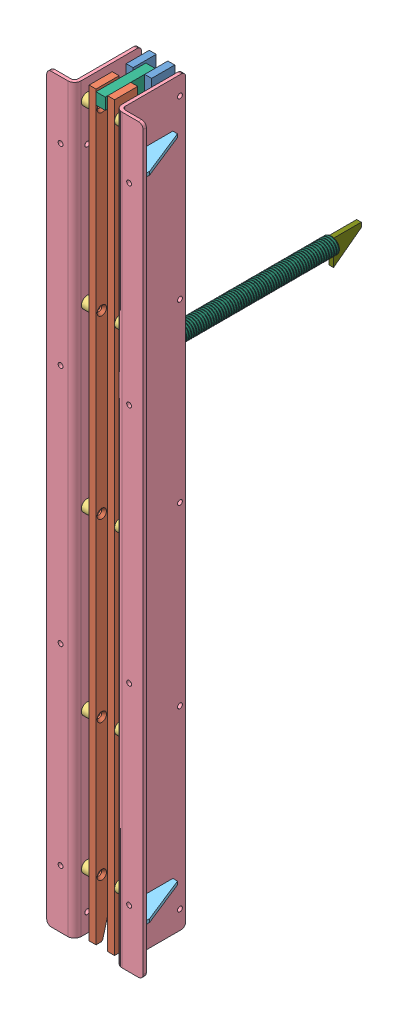
SolidWorks assembly GE-17046_ASM_34_ASM, configuration Default. Lengths in mm.
Overall size (132.08 1016 362.08).
57 component instances, 16 part files, 0 mates.
Components (placement in the parent):
- GE-17052_ASM_16_ASM-1: GE-17052_ASM_16_ASM [Default] at origin size (58.1 1016 92.08)
  - GE-17053_21-1: GE-17053_21 [Default] at origin size (9.53 1016 31.75)
  - GE-17054_26-1: GE-17054_26 [Default] at (9.525 1016 50.8) x (-1 0 0) z (0 0 1) size (9.53 1016 31.75)
  - GE-17057_10-1: GE-17057_10 [Default] at (20.0025 990.6 58.7375) x (-1 0 0) z (0 0 1) size (10.48 15.88 15.88)
  - GE-17057_10-2: GE-17057_10 [Default] at (9.525 25.4 -7.9375) size (10.48 15.88 15.88)
  - GE-17057_10-3: GE-17057_10 [Default] at (20.0025 749.3 58.7375) x (-1 0 0) z (0 0 1) size (10.48 15.88 15.88)
  - GE-17057_10-4: GE-17057_10 [Default] at (9.525 266.7 -7.9375) size (10.48 15.88 15.88)
  - GE-17057_10-5: GE-17057_10 [Default] at (20.0025 508 58.7375) x (-1 0 0) z (0 0 1) size (10.48 15.88 15.88)
  - GE-17057_10-6: GE-17057_10 [Default] at (9.525 508 -7.9375) size (10.48 15.88 15.88)
  - GE-17057_10-7: GE-17057_10 [Default] at (20.0025 266.7 58.7375) x (-1 0 0) z (0 0 1) size (10.48 15.88 15.88)
  - GE-17057_10-8: GE-17057_10 [Default] at (9.525 749.3 -7.9375) size (10.48 15.88 15.88)
  - GE-17057_10-9: GE-17057_10 [Default] at (20.0025 79.375 58.7375) x (-1 0 0) z (0 0 1) size (10.48 15.88 15.88)
  - GE-17057_10-10: GE-17057_10 [Default] at (9.525 990.6 -7.9375) size (10.48 15.88 15.88)
  - GE-17058_ASM_11_ASM-1: GE-17058_ASM_11_ASM [Default] at (20.0025 508 76.2) x (1 0 0) z (0 0 -1) size (38.1 1016 92.08)
    - GE-17058-01_19-1: GE-17058-01_19 [Default] at origin size (38.1 1016 92.08)
    - GE-17058-02_4-1: GE-17058-02_4 [Default] at (4.5542 -445.8792 4.5542) size (31.75 4.55 69.85)
    - GE-17058-02_4-2: GE-17058-02_4 [Default] at (4.5542 441.325 4.5542) size (31.75 4.55 69.85)
- GE-17047_ASM_25_ASM-1: GE-17047_ASM_25_ASM [Default] at (-1.5875 1014.4125 25.4) x (-1 0 0) z (0 0 1) size (49.23 520.7 354.14)
  - GE-17048_24-1: GE-17048_24 [Default] at origin size (12.7 520.7 85.73)
  - GE-17051_2-1: GE-17051_2 [Default] at (15.4686 179.3875 0) x (-1 0 0) z (0 0 1) size (2.77 9.53 9.53)
  - GE-17051_2-2: GE-17051_2 [Default] at (0 179.3875 0) x (-1 0 0) z (0 0 1) size (2.77 9.53 9.53)
  - GE-17050_3-1: GE-17050_3 [Default] at (15.4686 179.3875 0) size (4.98 15.88 15.88)
  - GE-17050_3-2: GE-17050_3 [Default] at (-7.747 179.3875 0) size (4.98 15.88 15.88)
  - HW-00501_2-1: HW-00501_2 [Default] at (23.7998 179.3875 0) x (0 1 0) z (1 0 0) size (11.17 11.22 39.58)
  - HW-00502_2_ASM-1: HW-00502_2_ASM [Default] at (-4.9784 179.3875 0) x (0 1 0) z (0 0 1) size (11.11 5.36 12.83)
    - MANIFOLD_SOLID_BREP_212996-1: MANIFOLD_SOLID_BREP_212996 [Default] at origin size (10.65 1.02 10.65)
    - MANIFOLD_SOLID_BREP_214924-1: MANIFOLD_SOLID_BREP_214924 [Default] at origin size (11.11 5.36 12.83)
  - GE-17051_2-3: GE-17051_2 [Default] at (15.4686 52.3875 0) x (-1 0 0) z (0 0 1) size (2.77 9.53 9.53)
  - GE-17051_2-4: GE-17051_2 [Default] at (0 52.3875 0) x (-1 0 0) z (0 0 1) size (2.77 9.53 9.53)
  - GE-17050_3-3: GE-17050_3 [Default] at (15.4686 52.3875 0) size (4.98 15.88 15.88)
  - GE-17050_3-4: GE-17050_3 [Default] at (-7.747 52.3875 0) size (4.98 15.88 15.88)
  - GE-17056_5-1: GE-17056_5 [Default] at (20.447 52.3875 0) size (4.76 9.53 9.53)
  - GE-17056_5-2: GE-17056_5 [Default] at (-12.5095 52.3875 0) size (4.76 9.53 9.53)
  - HW-00502_2_ASM-2: HW-00502_2_ASM [Default] at (-9.7409 52.3875 0) x (0 1 0) z (0 0 1) size (11.11 5.36 12.83)
    - MANIFOLD_SOLID_BREP_212996-1: MANIFOLD_SOLID_BREP_212996 [Default] at origin size (10.65 1.02 10.65)
    - MANIFOLD_SOLID_BREP_214924-1: MANIFOLD_SOLID_BREP_214924 [Default] at origin size (11.11 5.36 12.83)
  - HW-00505_3-1: HW-00505_3 [Default] at (28.5623 52.3875 0) x (0 1 0) z (1 0 0) size (11.17 11.22 49.23)
  - GE-17061_4-1: GE-17061_4 [Default] at (6.35 336.55 -42.8625) x (0 0 -1) z (0 1 0) size (25.4 16.76 16.76)
  - GE-17063_8-1: GE-17063_8 [Default] at (6.35 336.55 -44.577) x (0 -1 0) z (1 0 0) size (24.74 232.22 24.75)
  - GE-17064_6-1: GE-17064_6 [Default] at (6.35 336.55 -247.777) x (-1 0 0) z (0 0 -1) size (18.8 34.93 63.5)
- GE-17059_ASM_11_ASM-1: GE-17059_ASM_11_ASM [Default] at (-35.8775 508 76.2) x (1 0 0) z (0 0 -1) size (58.1 1016 92.08)
  - GE-17058_ASM_11_ASM-1: GE-17058_ASM_11_ASM [Default] x (-1 0 0) z (0 0 1) size (38.1 1016 92.08)
    - GE-17058-01_19-1: GE-17058-01_19 [Default] at origin size (38.1 1016 92.08)
    - GE-17058-02_4-1: GE-17058-02_4 [Default] at (4.5542 -445.8792 4.5542) size (31.75 4.55 69.85)
    - GE-17058-02_4-2: GE-17058-02_4 [Default] at (4.5542 441.325 4.5542) size (31.75 4.55 69.85)
  - GE-17057_10-1: GE-17057_10 [Default] at (0 -482.6 84.1375) size (10.48 15.88 15.88)
  - GE-17057_10-2: GE-17057_10 [Default] at (0 -482.6 17.4625) size (10.48 15.88 15.88)
  - GE-17057_10-3: GE-17057_10 [Default] at (0 -241.3 17.4625) size (10.48 15.88 15.88)
  - GE-17057_10-4: GE-17057_10 [Default] at (0 -241.3 84.1375) size (10.48 15.88 15.88)
  - GE-17057_10-5: GE-17057_10 [Default] at (0 0 17.4625) size (10.48 15.88 15.88)
  - GE-17057_10-6: GE-17057_10 [Default] at (0 0 84.1375) size (10.48 15.88 15.88)
  - GE-17057_10-7: GE-17057_10 [Default] at (0 241.3 17.4625) size (10.48 15.88 15.88)
  - GE-17057_10-8: GE-17057_10 [Default] at (0 241.3 84.1375) size (10.48 15.88 15.88)
  - GE-17057_10-9: GE-17057_10 [Default] at (0 428.625 17.4625) size (10.48 15.88 15.88)
  - GE-17057_10-10: GE-17057_10 [Default] at (0 482.6 84.1375) size (10.48 15.88 15.88)
  - GE-17053_21-1: GE-17053_21 [Default] at (20.0025 -508 76.2) x (-1 0 0) z (0 0 -1) size (9.53 1016 31.75)
  - GE-17054_26-1: GE-17054_26 [Default] at (20.0025 -508 25.4) x (-1 0 0) z (0 0 -1) size (9.53 1016 31.75)
